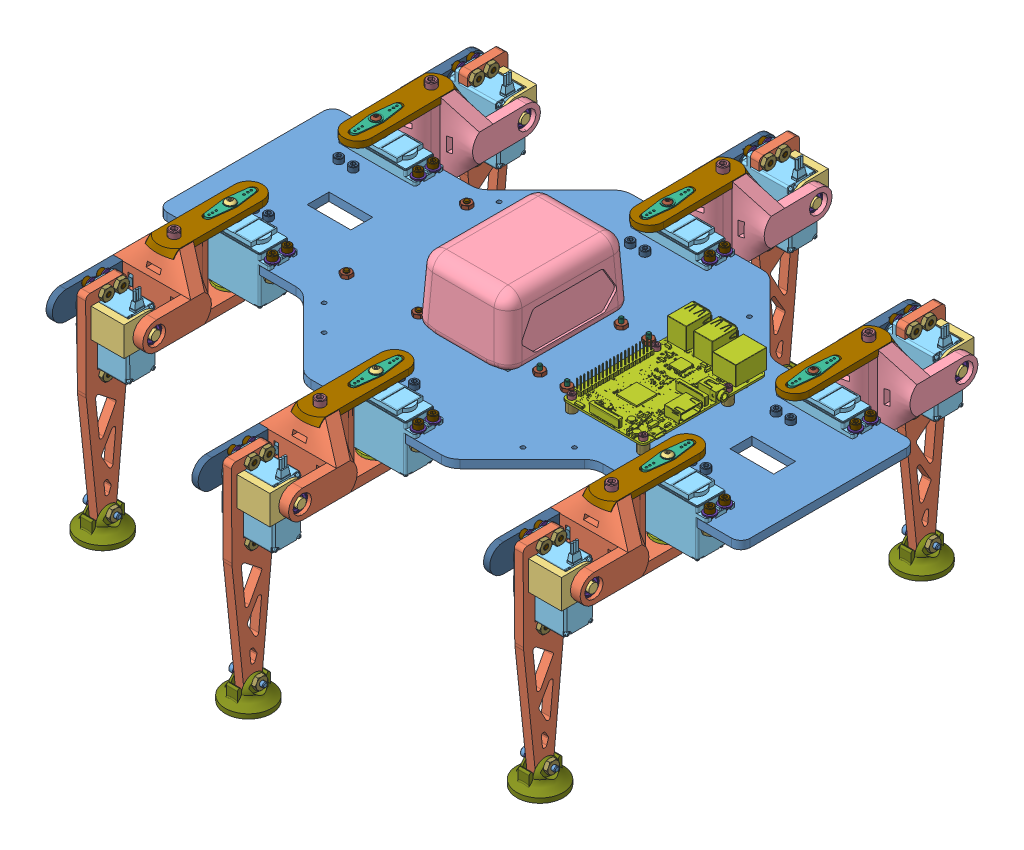
SolidWorks assembly Hexapod, configuration Défaut. Lengths in mm.
Overall size (400 185.52 400.77).
362 component instances, 31 part files, 135 mates.
Components (placement in the parent):
- Body-1: Body [Default] at (-400 -5.6 40) x (1 0 0) z (0 1 0) size (400 220 5.6)
- Leg_(Straight_Foot)-1: Leg_(Straight_Foot) [Default] at (-69.94 -26.67 -0.094) size (71.21 162.26 125.97)
  - Foot_(Straight)-1: Foot_(Straight) [Default] at (4.9357 4.6704 -91.3697) x (0.014203 -0.004273 0.99989) z (-0.999899 0 0.014203) size (28 145.4 6)
  - bearing_mount_foot-1: bearing_mount_foot [Default] at (4.8169 16.6442 -99.7278) x (-0.014203 0.004273 -0.99989) z (0.999899 0 -0.014203) size (25 20 29.5)
  - Joint-1: Joint [Défaut] at (35.768 26.4662 -54.7315) x (-0.014203 0 -0.999899) z (0 1 0) size (96.52 53.26 53.26)
  - hs-422-2: hs-422 [Défaut] at (5.1023 6.612 -77.4562) x (-0.014203 0.004273 -0.99989) z (0.000061 0.999991 0.004272) size (19.81 42.09 58.23)
  - hs-422-3: hs-422 [Défaut] at (19.939 20.701 -19.812) x (0 0 1) z (-1 0 0) size (19.81 42.09 58.23)
  - hs-422_horn_straight-1: hs-422_horn_straight [Default] at (-16.9088 16.9412 -87.0065) x (0.014203 0 0.999899) z (0 1 0) size (33.93 4.93 8.79)
  - hs-422_horn_straight-2: hs-422_horn_straight [Default] at (9.652 42.5743 -9.906) x (-0.014203 0 -0.999899) z (-0.999899 0 0.014203) size (33.93 4.93 8.79)
  - Bearing_mount_leg-1: Bearing_mount_leg [Default] at (9.652 21 2.594) x (0 0 1) z (0 -1 0) size (35 20 30)
  - Bearing-1: Bearing [Default] at (9.652 -6.7498 -9.906) x (0.84763 0 0.530588) z (-0.530588 0 0.84763) size (13.87 4.75 13.87)
  - Bearing-2: Bearing [Default] at (32.2403 16.9412 -87.7047) x (0.007588 -0.845349 0.534161) z (-0.012007 -0.534214 -0.845264) size (13.87 4.75 13.87)
  - Joint_attachment_leg-1: Joint_attachment_leg [Défaut] at (35.768 26.4662 -54.7315) x (-0.014203 0 -0.999899) z (0 1 0) size (74.32 19.07 4.32)
  - Joint_attachment_foot-1: Joint_attachment_foot [Défaut] at (35.768 26.4662 -54.7315) x (-0.014203 0 -0.999899) z (0 1 0) size (64.08 6.7 19.07)
  - SBHCSCREW 0.112-40x0.25-HX-N-2: SBHCSCREW 0.112-40x0.25-HX-N [SBHCSCREW 0.112-40x0.25-HX-N] at (-19.9057 16.9412 -86.964) x (0.999899 0 -0.014203) z (-0.007102 0.866025 -0.49995) size (7.85 5.41 5.41)
  - SBHCSCREW 0.112-40x0.25-HX-N-3: SBHCSCREW 0.112-40x0.25-HX-N [SBHCSCREW 0.112-40x0.25-HX-N] at (9.652 45.5715 -9.906) x (0 -1 0) z (0.87304 0 0.487649) size (7.85 5.41 5.41)
  - MSHXNUT 0.138-32-D-N-15: MSHXNUT 0.138-32-D-N [MSHXNUT 0.138-32-D-N] at (5.0634 -17.1179 -82.3793) x (0.012331 0.496295 0.868066) z (-0.999899 0 0.014203) size (7.92 9.15 2.9)
  - MSHXNUT 0.138-32-D-N-16: MSHXNUT 0.138-32-D-N [MSHXNUT 0.138-32-D-N] at (4.9191 -17.0756 -92.5381) x (-0.01227 0.503696 -0.863794) z (-0.999899 0 0.014203) size (7.92 9.15 2.9)
  - MSHXNUT 0.138-32-D-N-17: MSHXNUT 0.138-32-D-N [MSHXNUT 0.138-32-D-N] at (5.0662 30.3817 -82.1827) x (0.000061 0.999991 0.004272) z (-0.999899 0 0.014203) size (7.92 9.15 2.9)
  - MSHXNUT 0.138-32-D-N-18: MSHXNUT 0.138-32-D-N [MSHXNUT 0.138-32-D-N] at (4.9219 30.4239 -92.3416) x (0.000061 0.999991 0.004272) z (-0.999899 0 0.014203) size (7.92 9.15 2.9)
  - HX-SHCS 0.164-32x0.5x0.5-N-1: HX-SHCS 0.164-32x0.5x0.5-N [HX-SHCS 0.164-32x0.5x0.5-N] at (9.1052 47.8568 -48.4) x (0 -1 0) z (0.014203 0 0.999899) size (16.87 6.86 6.86)
  - HX-SHCS 0.164-32x0.5x0.5-N-2: HX-SHCS 0.164-32x0.5x0.5-N [HX-SHCS 0.164-32x0.5x0.5-N] at (-21.967 16.9412 -59.205) x (0.999899 0 -0.014203) z (0.014203 0 0.999899) size (16.87 6.86 6.86)
  - MSHXNUT 0.164-32-D-N-11: MSHXNUT 0.164-32-D-N [MSHXNUT 0.164-32-D-N] at (9.1052 33.127 -48.4) x (0.87304 0 0.487649) z (0 1 0) size (8.74 10.09 3.3)
  - MSHXNUT 0.164-32-D-N-12: MSHXNUT 0.164-32-D-N [MSHXNUT 0.164-32-D-N] at (-7.2387 16.9412 -59.4142) x (0.014203 0 0.999899) z (-0.999899 0 0.014203) size (8.74 10.09 3.3)
  - HX-SHCS 0.112-40x0.5x0.5-N-7: HX-SHCS 0.112-40x0.5x0.5-N [HX-SHCS 0.112-40x0.5x0.5-N] at (-4.0273 11.7063 -99.6232) x (0.999899 0 -0.014203) z (0.014203 -0.004273 0.99989) size (15.54 4.65 4.65)
  - HX-SHCS 0.112-40x0.5x0.5-N-8: HX-SHCS 0.112-40x0.5x0.5-N [HX-SHCS 0.112-40x0.5x0.5-N] at (-4.0267 21.7062 -99.5805) x (0.999899 0 -0.014203) z (-0.014203 0.004273 -0.99989) size (15.54 4.65 4.65)
  - Slippers-1: Slippers [Default] at (1.9296 -111.2294 -91.7731) x (0.999899 0 -0.014203) z (0.014203 0 0.999899) size (35.48 18.25 37.71)
  - Narrow FW 0.138-1: Narrow FW 0.138 [Narrow FW 0.138] at (-3.4475 30.3814 -82.0597) x (0.999899 0 -0.014203) z (0.014203 0 0.999899) size (0.81 7.92 7.92)
  - HX-SHCS 0.138-32x0.5x0.5-N-2: HX-SHCS 0.138-32x0.5x0.5-N [HX-SHCS 0.138-32x0.5x0.5-N] at (-8.0191 30.3814 -81.9948) x (0.999899 0 -0.014203) z (0.014203 0 0.999899) size (16.21 5.74 5.74)
  - Narrow FW 0.138-2: Narrow FW 0.138 [Narrow FW 0.138] at (-3.4504 -17.1182 -82.2627) x (0.999899 0 -0.014203) z (0.014203 0 0.999899) size (0.81 7.92 7.92)
  - Narrow FW 0.138-3: Narrow FW 0.138 [Narrow FW 0.138] at (-3.5919 30.4248 -92.2186) x (0.999899 0 -0.014203) z (0.014203 0 0.999899) size (0.81 7.92 7.92)
  - Narrow FW 0.138-4: Narrow FW 0.138 [Narrow FW 0.138] at (-3.5947 -17.0748 -92.4216) x (0.999899 0 -0.014203) z (0.014203 0 0.999899) size (0.81 7.92 7.92)
  - HX-SHCS 0.138-32x0.5x0.5-N-3: HX-SHCS 0.138-32x0.5x0.5-N [HX-SHCS 0.138-32x0.5x0.5-N] at (-8.022 -17.1182 -82.1977) x (0.999899 0 -0.014203) z (0.014203 0 0.999899) size (16.21 5.74 5.74)
  - HX-SHCS 0.138-32x0.5x0.5-N-4: HX-SHCS 0.138-32x0.5x0.5-N [HX-SHCS 0.138-32x0.5x0.5-N] at (-8.1634 30.4248 -92.1537) x (0.999899 0 -0.014203) z (0.014203 0 0.999899) size (16.21 5.74 5.74)
  - HX-SHCS 0.138-32x0.5x0.5-N-5: HX-SHCS 0.138-32x0.5x0.5-N [HX-SHCS 0.138-32x0.5x0.5-N] at (-8.1663 -17.0748 -92.3566) x (0.999899 0 -0.014203) z (0.014203 0 0.999899) size (16.21 5.74 5.74)
  - HX-SHCS 0.138-32x0.5x0.5-N-6: HX-SHCS 0.138-32x0.5x0.5-N [HX-SHCS 0.138-32x0.5x0.5-N] at (-3.81 33.7566 -14.986) x (0 -1 0) z (-0.55878 0 0.829316) size (16.21 5.74 5.74)
  - Narrow FW 0.138-5: Narrow FW 0.138 [Narrow FW 0.138] at (-3.81 29.1846 -14.986) x (0 -1 0) z (0.55878 0 -0.829316) size (0.81 7.92 7.92)
  - Narrow FW 0.138-6: Narrow FW 0.138 [Narrow FW 0.138] at (43.69 29.1846 -14.986) x (0 -1 0) z (0.55878 0 -0.829316) size (0.81 7.92 7.92)
  - Narrow FW 0.138-7: Narrow FW 0.138 [Narrow FW 0.138] at (-3.81 29.1846 -4.826) x (0 -1 0) z (0.55878 0 -0.829316) size (0.81 7.92 7.92)
  - Narrow FW 0.138-8: Narrow FW 0.138 [Narrow FW 0.138] at (43.69 29.1846 -4.826) x (0 -1 0) z (0.55878 0 -0.829316) size (0.81 7.92 7.92)
  - HX-SHCS 0.138-32x0.5x0.5-N-7: HX-SHCS 0.138-32x0.5x0.5-N [HX-SHCS 0.138-32x0.5x0.5-N] at (43.69 33.7566 -14.986) x (0 -1 0) z (-0.55878 0 0.829316) size (16.21 5.74 5.74)
  - HX-SHCS 0.138-32x0.5x0.5-N-8: HX-SHCS 0.138-32x0.5x0.5-N [HX-SHCS 0.138-32x0.5x0.5-N] at (-3.81 33.7566 -4.826) x (0 -1 0) z (-0.55878 0 0.829316) size (16.21 5.74 5.74)
  - HX-SHCS 0.138-32x0.5x0.5-N-9: HX-SHCS 0.138-32x0.5x0.5-N [HX-SHCS 0.138-32x0.5x0.5-N] at (43.69 33.7566 -4.826) x (0 -1 0) z (-0.55878 0 0.829316) size (16.21 5.74 5.74)
  - HX-SHCS 0.138-32x0.75x0.75-N-10: HX-SHCS 0.138-32x0.75x0.75-N [HX-SHCS 0.138-32x0.75x0.75-N] at (-8.9913 -99.7294 -91.618) x (0.999899 0 -0.014203) z (-0.012539 -0.46966 -0.882758) size (22.56 5.74 5.74)
  - Narrow FW 0.138-10: Narrow FW 0.138 [Narrow FW 0.138] at (-5.2324 -99.7294 -91.6714) x (-0.999899 0 0.014203) z (-0.011665 -0.570502 -0.821213) size (0.81 7.92 7.92)
  - MSHXNUT 0.138-32-D-N-19: MSHXNUT 0.138-32-D-N [MSHXNUT 0.138-32-D-N] at (8.279 -99.7294 -91.8633) x (0 1 0) z (-0.999899 0 0.014203) size (7.92 9.15 2.9)
- Leg_(Straight_Foot)-2: Leg_(Straight_Foot) [Default] at (-369.94 -26.67 -0.094) size (71.21 162.26 125.97)
  - Foot_(Straight)-1: Foot_(Straight) [Default] at (4.9357 4.6704 -91.3697) x (0.014203 -0.004273 0.99989) z (-0.999899 0 0.014203) size (28 145.4 6)
  - bearing_mount_foot-1: bearing_mount_foot [Default] at (4.8169 16.6442 -99.7278) x (-0.014203 0.004273 -0.99989) z (0.999899 0 -0.014203) size (25 20 29.5)
  - Joint-1: Joint [Défaut] at (35.768 26.4662 -54.7315) x (-0.014203 0 -0.999899) z (0 1 0) size (96.52 53.26 53.26)
  - hs-422-2: hs-422 [Défaut] at (5.1023 6.612 -77.4562) x (-0.014203 0.004273 -0.99989) z (0.000061 0.999991 0.004272) size (19.81 42.09 58.23)
  - hs-422-3: hs-422 [Défaut] at (19.939 20.701 -19.812) x (0 0 1) z (-1 0 0) size (19.81 42.09 58.23)
  - hs-422_horn_straight-1: hs-422_horn_straight [Default] at (-16.9088 16.9412 -87.0065) x (0.014203 0 0.999899) z (0 1 0) size (33.93 4.93 8.79)
  - hs-422_horn_straight-2: hs-422_horn_straight [Default] at (9.652 42.5743 -9.906) x (-0.014203 0 -0.999899) z (-0.999899 0 0.014203) size (33.93 4.93 8.79)
  - Bearing_mount_leg-1: Bearing_mount_leg [Default] at (9.652 21 2.594) x (0 0 1) z (0 -1 0) size (35 20 30)
  - Bearing-1: Bearing [Default] at (9.652 -6.7498 -9.906) x (0.84763 0 0.530588) z (-0.530588 0 0.84763) size (13.87 4.75 13.87)
  - Bearing-2: Bearing [Default] at (32.2403 16.9412 -87.7047) x (0.007588 -0.845349 0.534161) z (-0.012007 -0.534214 -0.845264) size (13.87 4.75 13.87)
  - Joint_attachment_leg-1: Joint_attachment_leg [Défaut] at (35.768 26.4662 -54.7315) x (-0.014203 0 -0.999899) z (0 1 0) size (74.32 19.07 4.32)
  - Joint_attachment_foot-1: Joint_attachment_foot [Défaut] at (35.768 26.4662 -54.7315) x (-0.014203 0 -0.999899) z (0 1 0) size (64.08 6.7 19.07)
  - SBHCSCREW 0.112-40x0.25-HX-N-2: SBHCSCREW 0.112-40x0.25-HX-N [SBHCSCREW 0.112-40x0.25-HX-N] at (-19.9057 16.9412 -86.964) x (0.999899 0 -0.014203) z (-0.007102 0.866025 -0.49995) size (7.85 5.41 5.41)
  - SBHCSCREW 0.112-40x0.25-HX-N-3: SBHCSCREW 0.112-40x0.25-HX-N [SBHCSCREW 0.112-40x0.25-HX-N] at (9.652 45.5715 -9.906) x (0 -1 0) z (0.87304 0 0.487649) size (7.85 5.41 5.41)
  - MSHXNUT 0.138-32-D-N-15: MSHXNUT 0.138-32-D-N [MSHXNUT 0.138-32-D-N] at (5.0634 -17.1179 -82.3793) x (0.012331 0.496295 0.868066) z (-0.999899 0 0.014203) size (7.92 9.15 2.9)
  - MSHXNUT 0.138-32-D-N-16: MSHXNUT 0.138-32-D-N [MSHXNUT 0.138-32-D-N] at (4.9191 -17.0756 -92.5381) x (-0.01227 0.503696 -0.863794) z (-0.999899 0 0.014203) size (7.92 9.15 2.9)
  - MSHXNUT 0.138-32-D-N-17: MSHXNUT 0.138-32-D-N [MSHXNUT 0.138-32-D-N] at (5.0662 30.3817 -82.1827) x (0.000061 0.999991 0.004272) z (-0.999899 0 0.014203) size (7.92 9.15 2.9)
  - MSHXNUT 0.138-32-D-N-18: MSHXNUT 0.138-32-D-N [MSHXNUT 0.138-32-D-N] at (4.9219 30.4239 -92.3416) x (0.000061 0.999991 0.004272) z (-0.999899 0 0.014203) size (7.92 9.15 2.9)
  - HX-SHCS 0.164-32x0.5x0.5-N-1: HX-SHCS 0.164-32x0.5x0.5-N [HX-SHCS 0.164-32x0.5x0.5-N] at (9.1052 47.8568 -48.4) x (0 -1 0) z (0.014203 0 0.999899) size (16.87 6.86 6.86)
  - HX-SHCS 0.164-32x0.5x0.5-N-2: HX-SHCS 0.164-32x0.5x0.5-N [HX-SHCS 0.164-32x0.5x0.5-N] at (-21.967 16.9412 -59.205) x (0.999899 0 -0.014203) z (0.014203 0 0.999899) size (16.87 6.86 6.86)
  - MSHXNUT 0.164-32-D-N-11: MSHXNUT 0.164-32-D-N [MSHXNUT 0.164-32-D-N] at (9.1052 33.127 -48.4) x (0.87304 0 0.487649) z (0 1 0) size (8.74 10.09 3.3)
  - MSHXNUT 0.164-32-D-N-12: MSHXNUT 0.164-32-D-N [MSHXNUT 0.164-32-D-N] at (-7.2387 16.9412 -59.4142) x (0.014203 0 0.999899) z (-0.999899 0 0.014203) size (8.74 10.09 3.3)
  - HX-SHCS 0.112-40x0.5x0.5-N-7: HX-SHCS 0.112-40x0.5x0.5-N [HX-SHCS 0.112-40x0.5x0.5-N] at (-4.0273 11.7063 -99.6232) x (0.999899 0 -0.014203) z (0.014203 -0.004273 0.99989) size (15.54 4.65 4.65)
  - HX-SHCS 0.112-40x0.5x0.5-N-8: HX-SHCS 0.112-40x0.5x0.5-N [HX-SHCS 0.112-40x0.5x0.5-N] at (-4.0267 21.7062 -99.5805) x (0.999899 0 -0.014203) z (-0.014203 0.004273 -0.99989) size (15.54 4.65 4.65)
  - Slippers-1: Slippers [Default] at (1.9296 -111.2294 -91.7731) x (0.999899 0 -0.014203) z (0.014203 0 0.999899) size (35.48 18.25 37.71)
  - Narrow FW 0.138-1: Narrow FW 0.138 [Narrow FW 0.138] at (-3.4475 30.3814 -82.0597) x (0.999899 0 -0.014203) z (0.014203 0 0.999899) size (0.81 7.92 7.92)
  - HX-SHCS 0.138-32x0.5x0.5-N-2: HX-SHCS 0.138-32x0.5x0.5-N [HX-SHCS 0.138-32x0.5x0.5-N] at (-8.0191 30.3814 -81.9948) x (0.999899 0 -0.014203) z (0.014203 0 0.999899) size (16.21 5.74 5.74)
  - Narrow FW 0.138-2: Narrow FW 0.138 [Narrow FW 0.138] at (-3.4504 -17.1182 -82.2627) x (0.999899 0 -0.014203) z (0.014203 0 0.999899) size (0.81 7.92 7.92)
  - Narrow FW 0.138-3: Narrow FW 0.138 [Narrow FW 0.138] at (-3.5919 30.4248 -92.2186) x (0.999899 0 -0.014203) z (0.014203 0 0.999899) size (0.81 7.92 7.92)
  - Narrow FW 0.138-4: Narrow FW 0.138 [Narrow FW 0.138] at (-3.5947 -17.0748 -92.4216) x (0.999899 0 -0.014203) z (0.014203 0 0.999899) size (0.81 7.92 7.92)
  - HX-SHCS 0.138-32x0.5x0.5-N-3: HX-SHCS 0.138-32x0.5x0.5-N [HX-SHCS 0.138-32x0.5x0.5-N] at (-8.022 -17.1182 -82.1977) x (0.999899 0 -0.014203) z (0.014203 0 0.999899) size (16.21 5.74 5.74)
  - HX-SHCS 0.138-32x0.5x0.5-N-4: HX-SHCS 0.138-32x0.5x0.5-N [HX-SHCS 0.138-32x0.5x0.5-N] at (-8.1634 30.4248 -92.1537) x (0.999899 0 -0.014203) z (0.014203 0 0.999899) size (16.21 5.74 5.74)
  - HX-SHCS 0.138-32x0.5x0.5-N-5: HX-SHCS 0.138-32x0.5x0.5-N [HX-SHCS 0.138-32x0.5x0.5-N] at (-8.1663 -17.0748 -92.3566) x (0.999899 0 -0.014203) z (0.014203 0 0.999899) size (16.21 5.74 5.74)
  - HX-SHCS 0.138-32x0.5x0.5-N-6: HX-SHCS 0.138-32x0.5x0.5-N [HX-SHCS 0.138-32x0.5x0.5-N] at (-3.81 33.7566 -14.986) x (0 -1 0) z (-0.55878 0 0.829316) size (16.21 5.74 5.74)
  - Narrow FW 0.138-5: Narrow FW 0.138 [Narrow FW 0.138] at (-3.81 29.1846 -14.986) x (0 -1 0) z (0.55878 0 -0.829316) size (0.81 7.92 7.92)
  - Narrow FW 0.138-6: Narrow FW 0.138 [Narrow FW 0.138] at (43.69 29.1846 -14.986) x (0 -1 0) z (0.55878 0 -0.829316) size (0.81 7.92 7.92)
  - Narrow FW 0.138-7: Narrow FW 0.138 [Narrow FW 0.138] at (-3.81 29.1846 -4.826) x (0 -1 0) z (0.55878 0 -0.829316) size (0.81 7.92 7.92)
  - Narrow FW 0.138-8: Narrow FW 0.138 [Narrow FW 0.138] at (43.69 29.1846 -4.826) x (0 -1 0) z (0.55878 0 -0.829316) size (0.81 7.92 7.92)
  - HX-SHCS 0.138-32x0.5x0.5-N-7: HX-SHCS 0.138-32x0.5x0.5-N [HX-SHCS 0.138-32x0.5x0.5-N] at (43.69 33.7566 -14.986) x (0 -1 0) z (-0.55878 0 0.829316) size (16.21 5.74 5.74)
  - HX-SHCS 0.138-32x0.5x0.5-N-8: HX-SHCS 0.138-32x0.5x0.5-N [HX-SHCS 0.138-32x0.5x0.5-N] at (-3.81 33.7566 -4.826) x (0 -1 0) z (-0.55878 0 0.829316) size (16.21 5.74 5.74)
  - HX-SHCS 0.138-32x0.5x0.5-N-9: HX-SHCS 0.138-32x0.5x0.5-N [HX-SHCS 0.138-32x0.5x0.5-N] at (43.69 33.7566 -4.826) x (0 -1 0) z (-0.55878 0 0.829316) size (16.21 5.74 5.74)
  - HX-SHCS 0.138-32x0.75x0.75-N-10: HX-SHCS 0.138-32x0.75x0.75-N [HX-SHCS 0.138-32x0.75x0.75-N] at (-8.9913 -99.7294 -91.618) x (0.999899 0 -0.014203) z (-0.012539 -0.46966 -0.882758) size (22.56 5.74 5.74)
  - Narrow FW 0.138-10: Narrow FW 0.138 [Narrow FW 0.138] at (-5.2324 -99.7294 -91.6714) x (-0.999899 0 0.014203) z (-0.011665 -0.570502 -0.821213) size (0.81 7.92 7.92)
  - MSHXNUT 0.138-32-D-N-19: MSHXNUT 0.138-32-D-N [MSHXNUT 0.138-32-D-N] at (8.279 -99.7294 -91.8633) x (0 1 0) z (-0.999899 0 0.014203) size (7.92 9.15 2.9)
- Leg_(Straight_Foot)-3: Leg_(Straight_Foot) [Default] at (-219.94 -26.67 -50.094) size (71.21 162.26 125.97)
  - Foot_(Straight)-1: Foot_(Straight) [Default] at (4.9357 4.6704 -91.3697) x (0.014203 -0.004273 0.99989) z (-0.999899 0 0.014203) size (28 145.4 6)
  - bearing_mount_foot-1: bearing_mount_foot [Default] at (4.8169 16.6442 -99.7278) x (-0.014203 0.004273 -0.99989) z (0.999899 0 -0.014203) size (25 20 29.5)
  - Joint-1: Joint [Défaut] at (35.768 26.4662 -54.7315) x (-0.014203 0 -0.999899) z (0 1 0) size (96.52 53.26 53.26)
  - hs-422-2: hs-422 [Défaut] at (5.1023 6.612 -77.4562) x (-0.014203 0.004273 -0.99989) z (0.000061 0.999991 0.004272) size (19.81 42.09 58.23)
  - hs-422-3: hs-422 [Défaut] at (19.939 20.701 -19.812) x (0 0 1) z (-1 0 0) size (19.81 42.09 58.23)
  - hs-422_horn_straight-1: hs-422_horn_straight [Default] at (-16.9088 16.9412 -87.0065) x (0.014203 0 0.999899) z (0 1 0) size (33.93 4.93 8.79)
  - hs-422_horn_straight-2: hs-422_horn_straight [Default] at (9.652 42.5743 -9.906) x (-0.014203 0 -0.999899) z (-0.999899 0 0.014203) size (33.93 4.93 8.79)
  - Bearing_mount_leg-1: Bearing_mount_leg [Default] at (9.652 21 2.594) x (0 0 1) z (0 -1 0) size (35 20 30)
  - Bearing-1: Bearing [Default] at (9.652 -6.7498 -9.906) x (0.84763 0 0.530588) z (-0.530588 0 0.84763) size (13.87 4.75 13.87)
  - Bearing-2: Bearing [Default] at (32.2403 16.9412 -87.7047) x (0.007588 -0.845349 0.534161) z (-0.012007 -0.534214 -0.845264) size (13.87 4.75 13.87)
  - Joint_attachment_leg-1: Joint_attachment_leg [Défaut] at (35.768 26.4662 -54.7315) x (-0.014203 0 -0.999899) z (0 1 0) size (74.32 19.07 4.32)
  - Joint_attachment_foot-1: Joint_attachment_foot [Défaut] at (35.768 26.4662 -54.7315) x (-0.014203 0 -0.999899) z (0 1 0) size (64.08 6.7 19.07)
  - SBHCSCREW 0.112-40x0.25-HX-N-2: SBHCSCREW 0.112-40x0.25-HX-N [SBHCSCREW 0.112-40x0.25-HX-N] at (-19.9057 16.9412 -86.964) x (0.999899 0 -0.014203) z (-0.007102 0.866025 -0.49995) size (7.85 5.41 5.41)
  - SBHCSCREW 0.112-40x0.25-HX-N-3: SBHCSCREW 0.112-40x0.25-HX-N [SBHCSCREW 0.112-40x0.25-HX-N] at (9.652 45.5715 -9.906) x (0 -1 0) z (0.87304 0 0.487649) size (7.85 5.41 5.41)
  - MSHXNUT 0.138-32-D-N-15: MSHXNUT 0.138-32-D-N [MSHXNUT 0.138-32-D-N] at (5.0634 -17.1179 -82.3793) x (0.012331 0.496295 0.868066) z (-0.999899 0 0.014203) size (7.92 9.15 2.9)
  - MSHXNUT 0.138-32-D-N-16: MSHXNUT 0.138-32-D-N [MSHXNUT 0.138-32-D-N] at (4.9191 -17.0756 -92.5381) x (-0.01227 0.503696 -0.863794) z (-0.999899 0 0.014203) size (7.92 9.15 2.9)
  - MSHXNUT 0.138-32-D-N-17: MSHXNUT 0.138-32-D-N [MSHXNUT 0.138-32-D-N] at (5.0662 30.3817 -82.1827) x (0.000061 0.999991 0.004272) z (-0.999899 0 0.014203) size (7.92 9.15 2.9)
  - MSHXNUT 0.138-32-D-N-18: MSHXNUT 0.138-32-D-N [MSHXNUT 0.138-32-D-N] at (4.9219 30.4239 -92.3416) x (0.000061 0.999991 0.004272) z (-0.999899 0 0.014203) size (7.92 9.15 2.9)
  - HX-SHCS 0.164-32x0.5x0.5-N-1: HX-SHCS 0.164-32x0.5x0.5-N [HX-SHCS 0.164-32x0.5x0.5-N] at (9.1052 47.8568 -48.4) x (0 -1 0) z (0.014203 0 0.999899) size (16.87 6.86 6.86)
  - HX-SHCS 0.164-32x0.5x0.5-N-2: HX-SHCS 0.164-32x0.5x0.5-N [HX-SHCS 0.164-32x0.5x0.5-N] at (-21.967 16.9412 -59.205) x (0.999899 0 -0.014203) z (0.014203 0 0.999899) size (16.87 6.86 6.86)
  - MSHXNUT 0.164-32-D-N-11: MSHXNUT 0.164-32-D-N [MSHXNUT 0.164-32-D-N] at (9.1052 33.127 -48.4) x (0.87304 0 0.487649) z (0 1 0) size (8.74 10.09 3.3)
  - MSHXNUT 0.164-32-D-N-12: MSHXNUT 0.164-32-D-N [MSHXNUT 0.164-32-D-N] at (-7.2387 16.9412 -59.4142) x (0.014203 0 0.999899) z (-0.999899 0 0.014203) size (8.74 10.09 3.3)
  - HX-SHCS 0.112-40x0.5x0.5-N-7: HX-SHCS 0.112-40x0.5x0.5-N [HX-SHCS 0.112-40x0.5x0.5-N] at (-4.0273 11.7063 -99.6232) x (0.999899 0 -0.014203) z (0.014203 -0.004273 0.99989) size (15.54 4.65 4.65)
  - HX-SHCS 0.112-40x0.5x0.5-N-8: HX-SHCS 0.112-40x0.5x0.5-N [HX-SHCS 0.112-40x0.5x0.5-N] at (-4.0267 21.7062 -99.5805) x (0.999899 0 -0.014203) z (-0.014203 0.004273 -0.99989) size (15.54 4.65 4.65)
  - Slippers-1: Slippers [Default] at (1.9296 -111.2294 -91.7731) x (0.999899 0 -0.014203) z (0.014203 0 0.999899) size (35.48 18.25 37.71)
  - Narrow FW 0.138-1: Narrow FW 0.138 [Narrow FW 0.138] at (-3.4475 30.3814 -82.0597) x (0.999899 0 -0.014203) z (0.014203 0 0.999899) size (0.81 7.92 7.92)
  - HX-SHCS 0.138-32x0.5x0.5-N-2: HX-SHCS 0.138-32x0.5x0.5-N [HX-SHCS 0.138-32x0.5x0.5-N] at (-8.0191 30.3814 -81.9948) x (0.999899 0 -0.014203) z (0.014203 0 0.999899) size (16.21 5.74 5.74)
  - Narrow FW 0.138-2: Narrow FW 0.138 [Narrow FW 0.138] at (-3.4504 -17.1182 -82.2627) x (0.999899 0 -0.014203) z (0.014203 0 0.999899) size (0.81 7.92 7.92)
  - Narrow FW 0.138-3: Narrow FW 0.138 [Narrow FW 0.138] at (-3.5919 30.4248 -92.2186) x (0.999899 0 -0.014203) z (0.014203 0 0.999899) size (0.81 7.92 7.92)
  - Narrow FW 0.138-4: Narrow FW 0.138 [Narrow FW 0.138] at (-3.5947 -17.0748 -92.4216) x (0.999899 0 -0.014203) z (0.014203 0 0.999899) size (0.81 7.92 7.92)
  - HX-SHCS 0.138-32x0.5x0.5-N-3: HX-SHCS 0.138-32x0.5x0.5-N [HX-SHCS 0.138-32x0.5x0.5-N] at (-8.022 -17.1182 -82.1977) x (0.999899 0 -0.014203) z (0.014203 0 0.999899) size (16.21 5.74 5.74)
  - HX-SHCS 0.138-32x0.5x0.5-N-4: HX-SHCS 0.138-32x0.5x0.5-N [HX-SHCS 0.138-32x0.5x0.5-N] at (-8.1634 30.4248 -92.1537) x (0.999899 0 -0.014203) z (0.014203 0 0.999899) size (16.21 5.74 5.74)
  - HX-SHCS 0.138-32x0.5x0.5-N-5: HX-SHCS 0.138-32x0.5x0.5-N [HX-SHCS 0.138-32x0.5x0.5-N] at (-8.1663 -17.0748 -92.3566) x (0.999899 0 -0.014203) z (0.014203 0 0.999899) size (16.21 5.74 5.74)
  - HX-SHCS 0.138-32x0.5x0.5-N-6: HX-SHCS 0.138-32x0.5x0.5-N [HX-SHCS 0.138-32x0.5x0.5-N] at (-3.81 33.7566 -14.986) x (0 -1 0) z (-0.55878 0 0.829316) size (16.21 5.74 5.74)
  - Narrow FW 0.138-5: Narrow FW 0.138 [Narrow FW 0.138] at (-3.81 29.1846 -14.986) x (0 -1 0) z (0.55878 0 -0.829316) size (0.81 7.92 7.92)
  - Narrow FW 0.138-6: Narrow FW 0.138 [Narrow FW 0.138] at (43.69 29.1846 -14.986) x (0 -1 0) z (0.55878 0 -0.829316) size (0.81 7.92 7.92)
  - Narrow FW 0.138-7: Narrow FW 0.138 [Narrow FW 0.138] at (-3.81 29.1846 -4.826) x (0 -1 0) z (0.55878 0 -0.829316) size (0.81 7.92 7.92)
  - Narrow FW 0.138-8: Narrow FW 0.138 [Narrow FW 0.138] at (43.69 29.1846 -4.826) x (0 -1 0) z (0.55878 0 -0.829316) size (0.81 7.92 7.92)
  - HX-SHCS 0.138-32x0.5x0.5-N-7: HX-SHCS 0.138-32x0.5x0.5-N [HX-SHCS 0.138-32x0.5x0.5-N] at (43.69 33.7566 -14.986) x (0 -1 0) z (-0.55878 0 0.829316) size (16.21 5.74 5.74)
  - HX-SHCS 0.138-32x0.5x0.5-N-8: HX-SHCS 0.138-32x0.5x0.5-N [HX-SHCS 0.138-32x0.5x0.5-N] at (-3.81 33.7566 -4.826) x (0 -1 0) z (-0.55878 0 0.829316) size (16.21 5.74 5.74)
  - HX-SHCS 0.138-32x0.5x0.5-N-9: HX-SHCS 0.138-32x0.5x0.5-N [HX-SHCS 0.138-32x0.5x0.5-N] at (43.69 33.7566 -4.826) x (0 -1 0) z (-0.55878 0 0.829316) size (16.21 5.74 5.74)
  - HX-SHCS 0.138-32x0.75x0.75-N-10: HX-SHCS 0.138-32x0.75x0.75-N [HX-SHCS 0.138-32x0.75x0.75-N] at (-8.9913 -99.7294 -91.618) x (0.999899 0 -0.014203) z (-0.012539 -0.46966 -0.882758) size (22.56 5.74 5.74)
  - Narrow FW 0.138-10: Narrow FW 0.138 [Narrow FW 0.138] at (-5.2324 -99.7294 -91.6714) x (-0.999899 0 0.014203) z (-0.011665 -0.570502 -0.821213) size (0.81 7.92 7.92)
  - MSHXNUT 0.138-32-D-N-19: MSHXNUT 0.138-32-D-N [MSHXNUT 0.138-32-D-N] at (8.279 -99.7294 -91.8633) x (0 1 0) z (-0.999899 0 0.014203) size (7.92 9.15 2.9)
- Leg_(Straight_Foot)_(Mirror)-1: Leg_(Straight_Foot)_(Mirror) [Default] at (-369.94 -26.67 99.906) size (70.36 162.3 124.8)
  - Joint_(Mirror)-1: Joint_(Mirror) [Défaut] at (36.4933 -51.1276 34.4889) x (0.002055 0 0.999998) z (0 -1 0) size (96.52 53.26 53.26)
  - hs-422-3: hs-422 [Défaut] at (19.939 20.701 -19.812) x (0 0 1) z (-1 0 0) size (19.81 42.09 58.23)
  - hs-422_horn_straight-2: hs-422_horn_straight [Default] at (9.652 42.5743 -9.906) x (0.002055 0 0.999998) z (0.999998 0 -0.002055) size (33.93 4.93 8.79)
  - Bearing_mount_leg-1: Bearing_mount_leg [Default] at (9.652 21 -22.406) x (0 0 -1) z (0 -1 0) size (35 20 30)
  - Bearing-1: Bearing [Default] at (9.652 -6.7498 -9.906) x (0.266287 0 0.963894) z (-0.963894 0 0.266287) size (13.87 4.75 13.87)
  - Joint_attachment_leg-1: Joint_attachment_leg [Défaut] at (-17.0066 26.5024 34.5989) x (0.002055 0 0.999998) z (0 1 0) size (74.32 19.07 4.32)
  - bearing_mount_foot-2: bearing_mount_foot [Default] at (6.7141 17.2663 79.9818) x (0.002055 -0.004919 0.999986) z (0.999998 0 -0.002055) size (25 20 29.5)
  - Bearing-3: Bearing [Default] at (29.1886 16.9774 67.524) x (-0.001098 -0.845349 -0.534213) z (0.001738 -0.534214 0.845347) size (13.87 4.75 13.87)
  - hs-422-4: hs-422 [Défaut] at (6.0779 6.6418 77.4268) x (-0.002055 0.004919 -0.999986) z (0.00001 0.999988 0.004919) size (19.81 42.09 58.23)
  - hs-422_horn_straight-3: hs-422_horn_straight [Default] at (-15.8156 16.9774 67.6165) x (-0.002055 0 -0.999998) z (0 -1 0) size (33.93 4.93 8.79)
  - Foot_(Straight)-2: Foot_(Straight) [Default] at (0.0967 4.6719 71.5233) x (-0.002055 0.004919 -0.999986) z (0.999998 0 -0.002055) size (28 145.4 6)
  - Joint_attachment_foot-2: Joint_attachment_foot [Défaut] at (36.4933 7.4524 34.4889) x (0.002055 0 0.999998) z (0 -1 0) size (64.08 6.7 19.07)
  - SBHCSCREW 0.138-32x0.25-HX-N-1: SBHCSCREW 0.138-32x0.25-HX-N [SBHCSCREW 0.138-32x0.25-HX-N] at (-19.1684 16.9774 67.6234) x (0.999998 0 -0.002055) z (0.002055 0 0.999998) size (8.2 6.65 6.65)
  - SBHCSCREW 0.138-32x0.25-HX-N-2: SBHCSCREW 0.138-32x0.25-HX-N [SBHCSCREW 0.138-32x0.25-HX-N] at (9.652 45.9271 -9.906) x (0 -1 0) z (-0.864996 0 0.501779) size (8.2 6.65 6.65)
  - HX-SHCS 0.112-40x0.5x0.5-N-5: HX-SHCS 0.112-40x0.5x0.5-N [HX-SHCS 0.112-40x0.5x0.5-N] at (-2.7306 21.6303 80.0227) x (0.999998 0 -0.002055) z (0.001019 -0.868474 0.495733) size (15.54 4.65 4.65)
  - HX-SHCS 0.112-40x0.5x0.5-N-6: HX-SHCS 0.112-40x0.5x0.5-N [HX-SHCS 0.112-40x0.5x0.5-N] at (-2.7307 11.6304 79.9735) x (0.999998 0 -0.002055) z (0.001036 0.863555 0.504253) size (15.54 4.65 4.65)
  - HX-SHCS 0.164-32x0.5x0.5-N-3: HX-SHCS 0.164-32x0.5x0.5-N [HX-SHCS 0.164-32x0.5x0.5-N] at (-21.1613 16.9774 39.9006) x (0.999998 0 -0.002055) z (0.001028 0.866025 0.499999) size (16.87 6.86 6.86)
  - HX-SHCS 0.164-32x0.5x0.5-N-4: HX-SHCS 0.164-32x0.5x0.5-N [HX-SHCS 0.164-32x0.5x0.5-N] at (9.7311 47.893 28.5918) x (0 -1 0) z (0.002055 0 0.999998) size (16.87 6.86 6.86)
  - MSHXNUT 0.138-32-D-N-14: MSHXNUT 0.138-32-D-N [MSHXNUT 0.138-32-D-N] at (6.0779 -17.0332 62.3241) x (-0.001785 -0.495734 -0.868473) z (-0.999998 0 0.002055) size (7.92 9.15 2.9)
  - MSHXNUT 0.138-32-D-N-15: MSHXNUT 0.138-32-D-N [MSHXNUT 0.138-32-D-N] at (8.9943 -17.0832 72.478) x (-0.001775 0.504254 -0.863554) z (0.999998 0 -0.002055) size (7.92 9.15 2.9)
  - MSHXNUT 0.138-32-D-N-16: MSHXNUT 0.138-32-D-N [MSHXNUT 0.138-32-D-N] at (8.9739 30.4662 62.5518) x (0.00001 0.999988 0.004919) z (0.999998 0 -0.002055) size (7.92 9.15 2.9)
  - MSHXNUT 0.138-32-D-N-17: MSHXNUT 0.138-32-D-N [MSHXNUT 0.138-32-D-N] at (6.0992 30.4162 72.7176) x (-0.001785 -0.495734 -0.868473) z (-0.999998 0 0.002055) size (7.92 9.15 2.9)
  - MSHXNUT 0.164-32-D-N-10: MSHXNUT 0.164-32-D-N [MSHXNUT 0.164-32-D-N] at (-6.4315 16.9774 39.8703) x (0.002055 0 0.999998) z (-0.999998 0 0.002055) size (8.74 10.09 3.3)
  - MSHXNUT 0.164-32-D-N-11: MSHXNUT 0.164-32-D-N [MSHXNUT 0.164-32-D-N] at (9.7311 29.8612 28.5918) x (-0.002055 0 -0.999998) z (0 -1 0) size (8.74 10.09 3.3)
  - Slippers-1: Slippers [Default] at (3.0957 -111.2276 71.0036) x (0.999998 0 -0.002055) z (0.002055 0 0.999998) size (35.48 18.25 37.71)
  - Narrow FW 0.138-4: Narrow FW 0.138 [Narrow FW 0.138] at (-2.4363 30.4642 62.5753) x (0.999998 0 -0.002055) z (0.002055 0 0.999998) size (0.81 7.92 7.92)
  - HX-SHCS 0.138-32x0.5x0.5-N-14: HX-SHCS 0.138-32x0.5x0.5-N [HX-SHCS 0.138-32x0.5x0.5-N] at (-7.0082 30.4642 62.5847) x (0.999998 0 -0.002055) z (0.002055 0 0.999998) size (16.21 5.74 5.74)
  - Narrow FW 0.138-5: Narrow FW 0.138 [Narrow FW 0.138] at (-2.4367 -17.0352 62.3416) x (0.999998 0 -0.002055) z (0.002055 0 0.999998) size (0.81 7.92 7.92)
  - Narrow FW 0.138-6: Narrow FW 0.138 [Narrow FW 0.138] at (-2.4154 30.4142 72.7351) x (0.999998 0 -0.002055) z (0.002055 0 0.999998) size (0.81 7.92 7.92)
  - Narrow FW 0.138-7: Narrow FW 0.138 [Narrow FW 0.138] at (-2.4158 -17.0852 72.5015) x (0.999998 0 -0.002055) z (0.002055 0 0.999998) size (0.81 7.92 7.92)
  - HX-SHCS 0.138-32x0.5x0.5-N-15: HX-SHCS 0.138-32x0.5x0.5-N [HX-SHCS 0.138-32x0.5x0.5-N] at (-7.0087 -17.0352 62.351) x (0.999998 0 -0.002055) z (0.002055 0 0.999998) size (16.21 5.74 5.74)
  - HX-SHCS 0.138-32x0.5x0.5-N-16: HX-SHCS 0.138-32x0.5x0.5-N [HX-SHCS 0.138-32x0.5x0.5-N] at (-6.9874 30.4142 72.7445) x (0.999998 0 -0.002055) z (0.002055 0 0.999998) size (16.21 5.74 5.74)
  - HX-SHCS 0.138-32x0.5x0.5-N-17: HX-SHCS 0.138-32x0.5x0.5-N [HX-SHCS 0.138-32x0.5x0.5-N] at (-6.9878 -17.0852 72.5109) x (0.999998 0 -0.002055) z (0.002055 0 0.999998) size (16.21 5.74 5.74)
  - Narrow FW 0.138-8: Narrow FW 0.138 [Narrow FW 0.138] at (-3.81 29.1846 -4.826) x (0 -1 0) z (0.55878 0 -0.829316) size (0.81 7.92 7.92)
  - HX-SHCS 0.138-32x0.5x0.5-N-18: HX-SHCS 0.138-32x0.5x0.5-N [HX-SHCS 0.138-32x0.5x0.5-N] at (-3.81 33.7566 -4.826) x (0 -1 0) z (-0.55878 0 0.829316) size (16.21 5.74 5.74)
  - Narrow FW 0.138-9: Narrow FW 0.138 [Narrow FW 0.138] at (43.69 29.1846 -4.826) x (0 -1 0) z (0.55878 0 -0.829316) size (0.81 7.92 7.92)
  - Narrow FW 0.138-10: Narrow FW 0.138 [Narrow FW 0.138] at (-3.81 29.1846 -14.986) x (0 -1 0) z (0.55878 0 -0.829316) size (0.81 7.92 7.92)
  - Narrow FW 0.138-11: Narrow FW 0.138 [Narrow FW 0.138] at (43.69 29.1846 -14.986) x (0 -1 0) z (0.55878 0 -0.829316) size (0.81 7.92 7.92)
  - HX-SHCS 0.138-32x0.5x0.5-N-19: HX-SHCS 0.138-32x0.5x0.5-N [HX-SHCS 0.138-32x0.5x0.5-N] at (43.69 33.7566 -4.826) x (0 -1 0) z (-0.55878 0 0.829316) size (16.21 5.74 5.74)
  - HX-SHCS 0.138-32x0.5x0.5-N-20: HX-SHCS 0.138-32x0.5x0.5-N [HX-SHCS 0.138-32x0.5x0.5-N] at (-3.81 33.7566 -14.986) x (0 -1 0) z (-0.55878 0 0.829316) size (16.21 5.74 5.74)
  - HX-SHCS 0.138-32x0.5x0.5-N-21: HX-SHCS 0.138-32x0.5x0.5-N [HX-SHCS 0.138-32x0.5x0.5-N] at (43.69 33.7566 -14.986) x (0 -1 0) z (-0.55878 0 0.829316) size (16.21 5.74 5.74)
  - HX-SHCS 0.138-32x0.75x0.75-N-1: HX-SHCS 0.138-32x0.75x0.75-N [HX-SHCS 0.138-32x0.75x0.75-N] at (-7.8263 -99.7276 71.0261) x (0.999998 0 -0.002055) z (-0.001815 -0.46966 -0.882845) size (22.56 5.74 5.74)
  - Narrow FW 0.138-12: Narrow FW 0.138 [Narrow FW 0.138] at (-4.0671 -99.7276 71.0183) x (-0.999998 0 0.002055) z (-0.001688 -0.570502 -0.821294) size (0.81 7.92 7.92)
  - MSHXNUT 0.138-32-D-N-18: MSHXNUT 0.138-32-D-N [MSHXNUT 0.138-32-D-N] at (9.4457 -99.7276 70.9906) x (0 1 0) z (-0.999998 0 0.002055) size (7.92 9.15 2.9)
- Leg_(Straight_Foot)_(Mirror)-2: Leg_(Straight_Foot)_(Mirror) [Default] at (-69.94 -26.67 99.906) size (70.36 162.3 124.8)
  - Joint_(Mirror)-1: Joint_(Mirror) [Défaut] at (36.4933 -51.1276 34.4889) x (0.002055 0 0.999998) z (0 -1 0) size (96.52 53.26 53.26)
  - hs-422-3: hs-422 [Défaut] at (19.939 20.701 -19.812) x (0 0 1) z (-1 0 0) size (19.81 42.09 58.23)
  - hs-422_horn_straight-2: hs-422_horn_straight [Default] at (9.652 42.5743 -9.906) x (0.002055 0 0.999998) z (0.999998 0 -0.002055) size (33.93 4.93 8.79)
  - Bearing_mount_leg-1: Bearing_mount_leg [Default] at (9.652 21 -22.406) x (0 0 -1) z (0 -1 0) size (35 20 30)
  - Bearing-1: Bearing [Default] at (9.652 -6.7498 -9.906) x (0.266287 0 0.963894) z (-0.963894 0 0.266287) size (13.87 4.75 13.87)
  - Joint_attachment_leg-1: Joint_attachment_leg [Défaut] at (-17.0066 26.5024 34.5989) x (0.002055 0 0.999998) z (0 1 0) size (74.32 19.07 4.32)
  - bearing_mount_foot-2: bearing_mount_foot [Default] at (6.7141 17.2663 79.9818) x (0.002055 -0.004919 0.999986) z (0.999998 0 -0.002055) size (25 20 29.5)
  - Bearing-3: Bearing [Default] at (29.1886 16.9774 67.524) x (-0.001098 -0.845349 -0.534213) z (0.001738 -0.534214 0.845347) size (13.87 4.75 13.87)
  - hs-422-4: hs-422 [Défaut] at (6.0779 6.6418 77.4268) x (-0.002055 0.004919 -0.999986) z (0.00001 0.999988 0.004919) size (19.81 42.09 58.23)
  - hs-422_horn_straight-3: hs-422_horn_straight [Default] at (-15.8156 16.9774 67.6165) x (-0.002055 0 -0.999998) z (0 -1 0) size (33.93 4.93 8.79)
  - Foot_(Straight)-2: Foot_(Straight) [Default] at (0.0967 4.6719 71.5233) x (-0.002055 0.004919 -0.999986) z (0.999998 0 -0.002055) size (28 145.4 6)
  - Joint_attachment_foot-2: Joint_attachment_foot [Défaut] at (36.4933 7.4524 34.4889) x (0.002055 0 0.999998) z (0 -1 0) size (64.08 6.7 19.07)
  - SBHCSCREW 0.138-32x0.25-HX-N-1: SBHCSCREW 0.138-32x0.25-HX-N [SBHCSCREW 0.138-32x0.25-HX-N] at (-19.1684 16.9774 67.6234) x (0.999998 0 -0.002055) z (0.002055 0 0.999998) size (8.2 6.65 6.65)
  - SBHCSCREW 0.138-32x0.25-HX-N-2: SBHCSCREW 0.138-32x0.25-HX-N [SBHCSCREW 0.138-32x0.25-HX-N] at (9.652 45.9271 -9.906) x (0 -1 0) z (-0.864996 0 0.501779) size (8.2 6.65 6.65)
  - HX-SHCS 0.112-40x0.5x0.5-N-5: HX-SHCS 0.112-40x0.5x0.5-N [HX-SHCS 0.112-40x0.5x0.5-N] at (-2.7306 21.6303 80.0227) x (0.999998 0 -0.002055) z (0.001019 -0.868474 0.495733) size (15.54 4.65 4.65)
  - HX-SHCS 0.112-40x0.5x0.5-N-6: HX-SHCS 0.112-40x0.5x0.5-N [HX-SHCS 0.112-40x0.5x0.5-N] at (-2.7307 11.6304 79.9735) x (0.999998 0 -0.002055) z (0.001036 0.863555 0.504253) size (15.54 4.65 4.65)
  - HX-SHCS 0.164-32x0.5x0.5-N-3: HX-SHCS 0.164-32x0.5x0.5-N [HX-SHCS 0.164-32x0.5x0.5-N] at (-21.1613 16.9774 39.9006) x (0.999998 0 -0.002055) z (0.001028 0.866025 0.499999) size (16.87 6.86 6.86)
  - HX-SHCS 0.164-32x0.5x0.5-N-4: HX-SHCS 0.164-32x0.5x0.5-N [HX-SHCS 0.164-32x0.5x0.5-N] at (9.7311 47.893 28.5918) x (0 -1 0) z (0.002055 0 0.999998) size (16.87 6.86 6.86)
  - MSHXNUT 0.138-32-D-N-14: MSHXNUT 0.138-32-D-N [MSHXNUT 0.138-32-D-N] at (6.0779 -17.0332 62.3241) x (-0.001785 -0.495734 -0.868473) z (-0.999998 0 0.002055) size (7.92 9.15 2.9)
  - MSHXNUT 0.138-32-D-N-15: MSHXNUT 0.138-32-D-N [MSHXNUT 0.138-32-D-N] at (8.9943 -17.0832 72.478) x (-0.001775 0.504254 -0.863554) z (0.999998 0 -0.002055) size (7.92 9.15 2.9)
  - MSHXNUT 0.138-32-D-N-16: MSHXNUT 0.138-32-D-N [MSHXNUT 0.138-32-D-N] at (8.9739 30.4662 62.5518) x (0.00001 0.999988 0.004919) z (0.999998 0 -0.002055) size (7.92 9.15 2.9)
  - MSHXNUT 0.138-32-D-N-17: MSHXNUT 0.138-32-D-N [MSHXNUT 0.138-32-D-N] at (6.0992 30.4162 72.7176) x (-0.001785 -0.495734 -0.868473) z (-0.999998 0 0.002055) size (7.92 9.15 2.9)
  - MSHXNUT 0.164-32-D-N-10: MSHXNUT 0.164-32-D-N [MSHXNUT 0.164-32-D-N] at (-6.4315 16.9774 39.8703) x (0.002055 0 0.999998) z (-0.999998 0 0.002055) size (8.74 10.09 3.3)
  - MSHXNUT 0.164-32-D-N-11: MSHXNUT 0.164-32-D-N [MSHXNUT 0.164-32-D-N] at (9.7311 29.8612 28.5918) x (-0.002055 0 -0.999998) z (0 -1 0) size (8.74 10.09 3.3)
  - Slippers-1: Slippers [Default] at (3.0957 -111.2276 71.0036) x (0.999998 0 -0.002055) z (0.002055 0 0.999998) size (35.48 18.25 37.71)
  - Narrow FW 0.138-4: Narrow FW 0.138 [Narrow FW 0.138] at (-2.4363 30.4642 62.5753) x (0.999998 0 -0.002055) z (0.002055 0 0.999998) size (0.81 7.92 7.92)
  - HX-SHCS 0.138-32x0.5x0.5-N-14: HX-SHCS 0.138-32x0.5x0.5-N [HX-SHCS 0.138-32x0.5x0.5-N] at (-7.0082 30.4642 62.5847) x (0.999998 0 -0.002055) z (0.002055 0 0.999998) size (16.21 5.74 5.74)
  - Narrow FW 0.138-5: Narrow FW 0.138 [Narrow FW 0.138] at (-2.4367 -17.0352 62.3416) x (0.999998 0 -0.002055) z (0.002055 0 0.999998) size (0.81 7.92 7.92)
  - Narrow FW 0.138-6: Narrow FW 0.138 [Narrow FW 0.138] at (-2.4154 30.4142 72.7351) x (0.999998 0 -0.002055) z (0.002055 0 0.999998) size (0.81 7.92 7.92)
  - Narrow FW 0.138-7: Narrow FW 0.138 [Narrow FW 0.138] at (-2.4158 -17.0852 72.5015) x (0.999998 0 -0.002055) z (0.002055 0 0.999998) size (0.81 7.92 7.92)
  - HX-SHCS 0.138-32x0.5x0.5-N-15: HX-SHCS 0.138-32x0.5x0.5-N [HX-SHCS 0.138-32x0.5x0.5-N] at (-7.0087 -17.0352 62.351) x (0.999998 0 -0.002055) z (0.002055 0 0.999998) size (16.21 5.74 5.74)
  - HX-SHCS 0.138-32x0.5x0.5-N-16: HX-SHCS 0.138-32x0.5x0.5-N [HX-SHCS 0.138-32x0.5x0.5-N] at (-6.9874 30.4142 72.7445) x (0.999998 0 -0.002055) z (0.002055 0 0.999998) size (16.21 5.74 5.74)
  - HX-SHCS 0.138-32x0.5x0.5-N-17: HX-SHCS 0.138-32x0.5x0.5-N [HX-SHCS 0.138-32x0.5x0.5-N] at (-6.9878 -17.0852 72.5109) x (0.999998 0 -0.002055) z (0.002055 0 0.999998) size (16.21 5.74 5.74)
  - Narrow FW 0.138-8: Narrow FW 0.138 [Narrow FW 0.138] at (-3.81 29.1846 -4.826) x (0 -1 0) z (0.55878 0 -0.829316) size (0.81 7.92 7.92)
  - HX-SHCS 0.138-32x0.5x0.5-N-18: HX-SHCS 0.138-32x0.5x0.5-N [HX-SHCS 0.138-32x0.5x0.5-N] at (-3.81 33.7566 -4.826) x (0 -1 0) z (-0.55878 0 0.829316) size (16.21 5.74 5.74)
  - Narrow FW 0.138-9: Narrow FW 0.138 [Narrow FW 0.138] at (43.69 29.1846 -4.826) x (0 -1 0) z (0.55878 0 -0.829316) size (0.81 7.92 7.92)
  - Narrow FW 0.138-10: Narrow FW 0.138 [Narrow FW 0.138] at (-3.81 29.1846 -14.986) x (0 -1 0) z (0.55878 0 -0.829316) size (0.81 7.92 7.92)
  - Narrow FW 0.138-11: Narrow FW 0.138 [Narrow FW 0.138] at (43.69 29.1846 -14.986) x (0 -1 0) z (0.55878 0 -0.829316) size (0.81 7.92 7.92)
  - HX-SHCS 0.138-32x0.5x0.5-N-19: HX-SHCS 0.138-32x0.5x0.5-N [HX-SHCS 0.138-32x0.5x0.5-N] at (43.69 33.7566 -4.826) x (0 -1 0) z (-0.55878 0 0.829316) size (16.21 5.74 5.74)
  - HX-SHCS 0.138-32x0.5x0.5-N-20: HX-SHCS 0.138-32x0.5x0.5-N [HX-SHCS 0.138-32x0.5x0.5-N] at (-3.81 33.7566 -14.986) x (0 -1 0) z (-0.55878 0 0.829316) size (16.21 5.74 5.74)
  - HX-SHCS 0.138-32x0.5x0.5-N-21: HX-SHCS 0.138-32x0.5x0.5-N [HX-SHCS 0.138-32x0.5x0.5-N] at (43.69 33.7566 -14.986) x (0 -1 0) z (-0.55878 0 0.829316) size (16.21 5.74 5.74)
  - HX-SHCS 0.138-32x0.75x0.75-N-1: HX-SHCS 0.138-32x0.75x0.75-N [HX-SHCS 0.138-32x0.75x0.75-N] at (-7.8263 -99.7276 71.0261) x (0.999998 0 -0.002055) z (-0.001815 -0.46966 -0.882845) size (22.56 5.74 5.74)
  - Narrow FW 0.138-12: Narrow FW 0.138 [Narrow FW 0.138] at (-4.0671 -99.7276 71.0183) x (-0.999998 0 0.002055) z (-0.001688 -0.570502 -0.821294) size (0.81 7.92 7.92)
  - MSHXNUT 0.138-32-D-N-18: MSHXNUT 0.138-32-D-N [MSHXNUT 0.138-32-D-N] at (9.4457 -99.7276 70.9906) x (0 1 0) z (-0.999998 0 0.002055) size (7.92 9.15 2.9)
- Leg_(Straight_Foot)_(Mirror)-3: Leg_(Straight_Foot)_(Mirror) [Default] at (-219.94 -26.67 149.906) size (70.36 162.3 124.8)
  - Joint_(Mirror)-1: Joint_(Mirror) [Défaut] at (36.4933 -51.1276 34.4889) x (0.002055 0 0.999998) z (0 -1 0) size (96.52 53.26 53.26)
  - hs-422-3: hs-422 [Défaut] at (19.939 20.701 -19.812) x (0 0 1) z (-1 0 0) size (19.81 42.09 58.23)
  - hs-422_horn_straight-2: hs-422_horn_straight [Default] at (9.652 42.5743 -9.906) x (0.002055 0 0.999998) z (0.999998 0 -0.002055) size (33.93 4.93 8.79)
  - Bearing_mount_leg-1: Bearing_mount_leg [Default] at (9.652 21 -22.406) x (0 0 -1) z (0 -1 0) size (35 20 30)
  - Bearing-1: Bearing [Default] at (9.652 -6.7498 -9.906) x (0.266287 0 0.963894) z (-0.963894 0 0.266287) size (13.87 4.75 13.87)
  - Joint_attachment_leg-1: Joint_attachment_leg [Défaut] at (-17.0066 26.5024 34.5989) x (0.002055 0 0.999998) z (0 1 0) size (74.32 19.07 4.32)
  - bearing_mount_foot-2: bearing_mount_foot [Default] at (6.7141 17.2663 79.9818) x (0.002055 -0.004919 0.999986) z (0.999998 0 -0.002055) size (25 20 29.5)
  - Bearing-3: Bearing [Default] at (29.1886 16.9774 67.524) x (-0.001098 -0.845349 -0.534213) z (0.001738 -0.534214 0.845347) size (13.87 4.75 13.87)
  - hs-422-4: hs-422 [Défaut] at (6.0779 6.6418 77.4268) x (-0.002055 0.004919 -0.999986) z (0.00001 0.999988 0.004919) size (19.81 42.09 58.23)
  - hs-422_horn_straight-3: hs-422_horn_straight [Default] at (-15.8156 16.9774 67.6165) x (-0.002055 0 -0.999998) z (0 -1 0) size (33.93 4.93 8.79)
  - Foot_(Straight)-2: Foot_(Straight) [Default] at (0.0967 4.6719 71.5233) x (-0.002055 0.004919 -0.999986) z (0.999998 0 -0.002055) size (28 145.4 6)
  - Joint_attachment_foot-2: Joint_attachment_foot [Défaut] at (36.4933 7.4524 34.4889) x (0.002055 0 0.999998) z (0 -1 0) size (64.08 6.7 19.07)
  - SBHCSCREW 0.138-32x0.25-HX-N-1: SBHCSCREW 0.138-32x0.25-HX-N [SBHCSCREW 0.138-32x0.25-HX-N] at (-19.1684 16.9774 67.6234) x (0.999998 0 -0.002055) z (0.002055 0 0.999998) size (8.2 6.65 6.65)
  - SBHCSCREW 0.138-32x0.25-HX-N-2: SBHCSCREW 0.138-32x0.25-HX-N [SBHCSCREW 0.138-32x0.25-HX-N] at (9.652 45.9271 -9.906) x (0 -1 0) z (-0.864996 0 0.501779) size (8.2 6.65 6.65)
  - HX-SHCS 0.112-40x0.5x0.5-N-5: HX-SHCS 0.112-40x0.5x0.5-N [HX-SHCS 0.112-40x0.5x0.5-N] at (-2.7306 21.6303 80.0227) x (0.999998 0 -0.002055) z (0.001019 -0.868474 0.495733) size (15.54 4.65 4.65)
  - HX-SHCS 0.112-40x0.5x0.5-N-6: HX-SHCS 0.112-40x0.5x0.5-N [HX-SHCS 0.112-40x0.5x0.5-N] at (-2.7307 11.6304 79.9735) x (0.999998 0 -0.002055) z (0.001036 0.863555 0.504253) size (15.54 4.65 4.65)
  - HX-SHCS 0.164-32x0.5x0.5-N-3: HX-SHCS 0.164-32x0.5x0.5-N [HX-SHCS 0.164-32x0.5x0.5-N] at (-21.1613 16.9774 39.9006) x (0.999998 0 -0.002055) z (0.001028 0.866025 0.499999) size (16.87 6.86 6.86)
  - HX-SHCS 0.164-32x0.5x0.5-N-4: HX-SHCS 0.164-32x0.5x0.5-N [HX-SHCS 0.164-32x0.5x0.5-N] at (9.7311 47.893 28.5918) x (0 -1 0) z (0.002055 0 0.999998) size (16.87 6.86 6.86)
  - MSHXNUT 0.138-32-D-N-14: MSHXNUT 0.138-32-D-N [MSHXNUT 0.138-32-D-N] at (6.0779 -17.0332 62.3241) x (-0.001785 -0.495734 -0.868473) z (-0.999998 0 0.002055) size (7.92 9.15 2.9)
  - MSHXNUT 0.138-32-D-N-15: MSHXNUT 0.138-32-D-N [MSHXNUT 0.138-32-D-N] at (8.9943 -17.0832 72.478) x (-0.001775 0.504254 -0.863554) z (0.999998 0 -0.002055) size (7.92 9.15 2.9)
  - MSHXNUT 0.138-32-D-N-16: MSHXNUT 0.138-32-D-N [MSHXNUT 0.138-32-D-N] at (8.9739 30.4662 62.5518) x (0.00001 0.999988 0.004919) z (0.999998 0 -0.002055) size (7.92 9.15 2.9)
  - MSHXNUT 0.138-32-D-N-17: MSHXNUT 0.138-32-D-N [MSHXNUT 0.138-32-D-N] at (6.0992 30.4162 72.7176) x (-0.001785 -0.495734 -0.868473) z (-0.999998 0 0.002055) size (7.92 9.15 2.9)
  - MSHXNUT 0.164-32-D-N-10: MSHXNUT 0.164-32-D-N [MSHXNUT 0.164-32-D-N] at (-6.4315 16.9774 39.8703) x (0.002055 0 0.999998) z (-0.999998 0 0.002055) size (8.74 10.09 3.3)
  - MSHXNUT 0.164-32-D-N-11: MSHXNUT 0.164-32-D-N [MSHXNUT 0.164-32-D-N] at (9.7311 29.8612 28.5918) x (-0.002055 0 -0.999998) z (0 -1 0) size (8.74 10.09 3.3)
  - Slippers-1: Slippers [Default] at (3.0957 -111.2276 71.0036) x (0.999998 0 -0.002055) z (0.002055 0 0.999998) size (35.48 18.25 37.71)
  - Narrow FW 0.138-4: Narrow FW 0.138 [Narrow FW 0.138] at (-2.4363 30.4642 62.5753) x (0.999998 0 -0.002055) z (0.002055 0 0.999998) size (0.81 7.92 7.92)
  - HX-SHCS 0.138-32x0.5x0.5-N-14: HX-SHCS 0.138-32x0.5x0.5-N [HX-SHCS 0.138-32x0.5x0.5-N] at (-7.0082 30.4642 62.5847) x (0.999998 0 -0.002055) z (0.002055 0 0.999998) size (16.21 5.74 5.74)
  - Narrow FW 0.138-5: Narrow FW 0.138 [Narrow FW 0.138] at (-2.4367 -17.0352 62.3416) x (0.999998 0 -0.002055) z (0.002055 0 0.999998) size (0.81 7.92 7.92)
  - Narrow FW 0.138-6: Narrow FW 0.138 [Narrow FW 0.138] at (-2.4154 30.4142 72.7351) x (0.999998 0 -0.002055) z (0.002055 0 0.999998) size (0.81 7.92 7.92)
  - Narrow FW 0.138-7: Narrow FW 0.138 [Narrow FW 0.138] at (-2.4158 -17.0852 72.5015) x (0.999998 0 -0.002055) z (0.002055 0 0.999998) size (0.81 7.92 7.92)
  - HX-SHCS 0.138-32x0.5x0.5-N-15: HX-SHCS 0.138-32x0.5x0.5-N [HX-SHCS 0.138-32x0.5x0.5-N] at (-7.0087 -17.0352 62.351) x (0.999998 0 -0.002055) z (0.002055 0 0.999998) size (16.21 5.74 5.74)
  - HX-SHCS 0.138-32x0.5x0.5-N-16: HX-SHCS 0.138-32x0.5x0.5-N [HX-SHCS 0.138-32x0.5x0.5-N] at (-6.9874 30.4142 72.7445) x (0.999998 0 -0.002055) z (0.002055 0 0.999998) size (16.21 5.74 5.74)
  - HX-SHCS 0.138-32x0.5x0.5-N-17: HX-SHCS 0.138-32x0.5x0.5-N [HX-SHCS 0.138-32x0.5x0.5-N] at (-6.9878 -17.0852 72.5109) x (0.999998 0 -0.002055) z (0.002055 0 0.999998) size (16.21 5.74 5.74)
  - Narrow FW 0.138-8: Narrow FW 0.138 [Narrow FW 0.138] at (-3.81 29.1846 -4.826) x (0 -1 0) z (0.55878 0 -0.829316) size (0.81 7.92 7.92)
  - HX-SHCS 0.138-32x0.5x0.5-N-18: HX-SHCS 0.138-32x0.5x0.5-N [HX-SHCS 0.138-32x0.5x0.5-N] at (-3.81 33.7566 -4.826) x (0 -1 0) z (-0.55878 0 0.829316) size (16.21 5.74 5.74)
  - Narrow FW 0.138-9: Narrow FW 0.138 [Narrow FW 0.138] at (43.69 29.1846 -4.826) x (0 -1 0) z (0.55878 0 -0.829316) size (0.81 7.92 7.92)
  - Narrow FW 0.138-10: Narrow FW 0.138 [Narrow FW 0.138] at (-3.81 29.1846 -14.986) x (0 -1 0) z (0.55878 0 -0.829316) size (0.81 7.92 7.92)
  - Narrow FW 0.138-11: Narrow FW 0.138 [Narrow FW 0.138] at (43.69 29.1846 -14.986) x (0 -1 0) z (0.55878 0 -0.829316) size (0.81 7.92 7.92)
  - HX-SHCS 0.138-32x0.5x0.5-N-19: HX-SHCS 0.138-32x0.5x0.5-N [HX-SHCS 0.138-32x0.5x0.5-N] at (43.69 33.7566 -4.826) x (0 -1 0) z (-0.55878 0 0.829316) size (16.21 5.74 5.74)
  - HX-SHCS 0.138-32x0.5x0.5-N-20: HX-SHCS 0.138-32x0.5x0.5-N [HX-SHCS 0.138-32x0.5x0.5-N] at (-3.81 33.7566 -14.986) x (0 -1 0) z (-0.55878 0 0.829316) size (16.21 5.74 5.74)
  - HX-SHCS 0.138-32x0.5x0.5-N-21: HX-SHCS 0.138-32x0.5x0.5-N [HX-SHCS 0.138-32x0.5x0.5-N] at (43.69 33.7566 -14.986) x (0 -1 0) z (-0.55878 0 0.829316) size (16.21 5.74 5.74)
  - HX-SHCS 0.138-32x0.75x0.75-N-1: HX-SHCS 0.138-32x0.75x0.75-N [HX-SHCS 0.138-32x0.75x0.75-N] at (-7.8263 -99.7276 71.0261) x (0.999998 0 -0.002055) z (-0.001815 -0.46966 -0.882845) size (22.56 5.74 5.74)
  - Narrow FW 0.138-12: Narrow FW 0.138 [Narrow FW 0.138] at (-4.0671 -99.7276 71.0183) x (-0.999998 0 0.002055) z (-0.001688 -0.570502 -0.821294) size (0.81 7.92 7.92)
  - MSHXNUT 0.138-32-D-N-18: MSHXNUT 0.138-32-D-N [MSHXNUT 0.138-32-D-N] at (9.4457 -99.7276 70.9906) x (0 1 0) z (-0.999998 0 0.002055) size (7.92 9.15 2.9)
